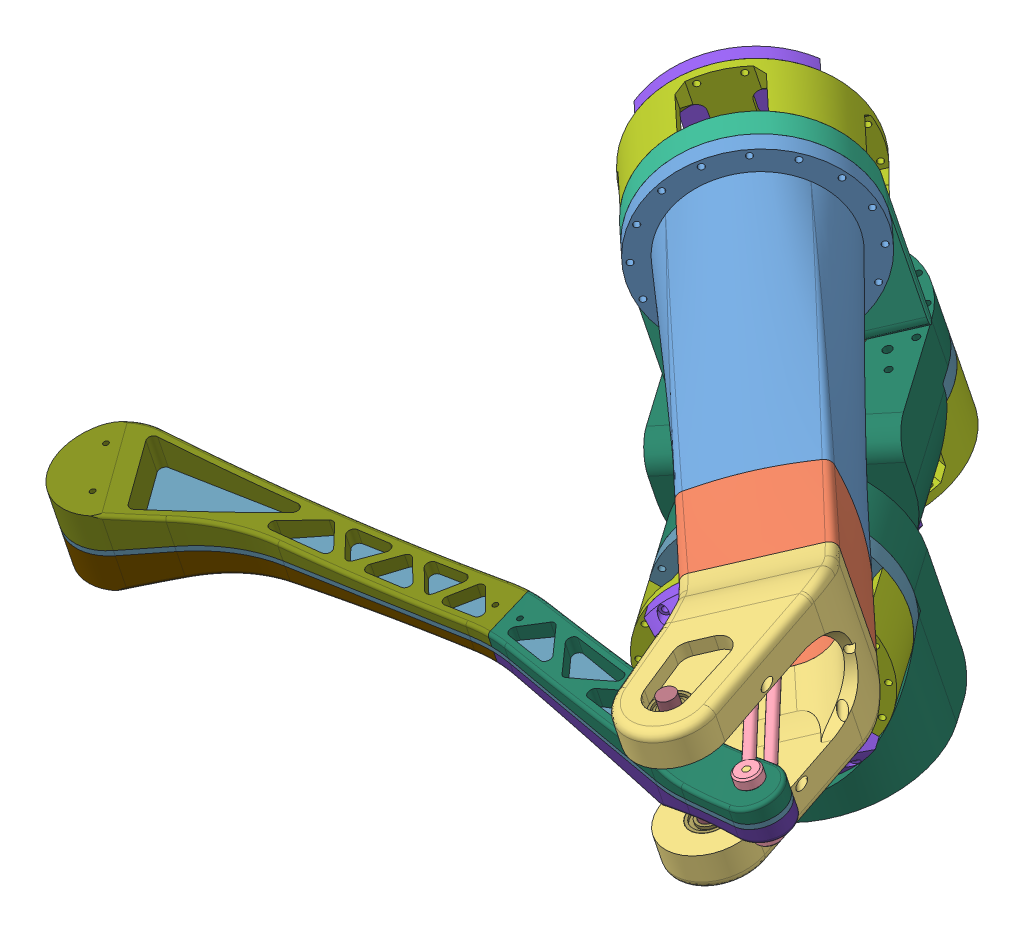
SolidWorks assembly Leg, configuration Default. Lengths in mm. (continued)
Components (placement in the parent): (continued)
- Cycloidal _v3-2: Cycloidal _v3 [Default] at (146.1775 22.9675 470.2476) x (0.670066 -0.524344 -0.525427) z (0.511404 0.83914 -0.185227) size (173.36 87.57 173.15) (continued)
  - foc-motor-controller.step-1: foc-motor-controller.step [Default] at (47.4677 32.6574 89.6282) x (0.701413 0.00028 0.712755) z (0.000399 -1 0) size (57.23 50 8.13) (continued)
    - C_1206_3216Metric.step-13: C_1206_3216Metric.step [Default] at (4 11 1.595) x (0 1 0) z (0 0 1) size (3.2 1.6 1.6)
    - R_0603_1608Metric.step-20: R_0603_1608Metric.step [Default] at (16 -17.8 1.595) x (0 1 0) z (0 0 1) size (1.6 0.8 0.45)
    - Texas_S-PVSON-N8.step-1: Texas_S-PVSON-N8.step [Default] at (-14.4105 -13.7 1.595) x (-1 0 0) z (0 0 1) size (3 2.98 0.92)
    - C_1206_3216Metric.step-14: C_1206_3216Metric.step [Default] at (21 -2.9 1.595) x (0.707107 -0.707107 0) z (0 0 1) size (3.2 1.6 1.6)
    - C_0603_1608Metric.step-24: C_0603_1608Metric.step [Default] at (-5.9 -16.6 1.595) x (0 1 0) z (0 0 1) size (1.6 0.8 0.8)
    - C_0603_1608Metric.step-25: C_0603_1608Metric.step [Default] at (-3.1 -14.1 1.595) size (1.6 0.8 0.8)
    - R_0603_1608Metric.step-21: R_0603_1608Metric.step [Default] at (7.2 -7.375 1.595) x (0 -1 0) z (0 0 1) size (1.6 0.8 0.45)
    - C_1206_3216Metric.step-15: C_1206_3216Metric.step [Default] at (-0.7 11 1.595) x (0 1 0) z (0 0 1) size (3.2 1.6 1.6)
    - LQFP-64_10x10mm_P0.5mm.step-1: LQFP-64_10x10mm_P0.5mm.step [Default] at (-7 -4.5 1.595) x (-1 0 0) z (0 0 1) size (12 12 1.5)
    - C_0805_2012Metric.step-2: C_0805_2012Metric.step [Default] at (23.35 -17 1.595) x (-1 0 0) z (0 0 1) size (2 1.25 1.25)
    - C_0603_1608Metric.step-26: C_0603_1608Metric.step [Default] at (10.8 -16.8 1.595) x (0 -1 0) z (0 0 1) size (1.6 0.8 0.8)
    - R_0603_1608Metric.step-22: R_0603_1608Metric.step [Default] at (17.5 -17.8 1.595) x (0 -1 0) z (0 0 1) size (1.6 0.8 0.45)
    - C_1206_3216Metric.step-16: C_1206_3216Metric.step [Default] at (20.3 11 1.595) x (0 1 0) z (0 0 1) size (3.2 1.6 1.6)
    - R_0603_1608Metric.step-23: R_0603_1608Metric.step [Default] at (9.2 -16.8 1.595) x (0 -1 0) z (0 0 1) size (1.6 0.8 0.45)
    - C_1206_3216Metric.step-17: C_1206_3216Metric.step [Default] at (-10 11 1.595) x (0 1 0) z (0 0 1) size (3.2 1.6 1.6)
    - R_0603_1608Metric.step-24: R_0603_1608Metric.step [Default] at (17.8 -15.2 1.595) size (1.6 0.8 0.45)
    - C_1206_3216Metric.step-18: C_1206_3216Metric.step [Default] at (19.9 2.6 1.595) x (-0.707107 0.707107 0) z (0 0 1) size (3.2 1.6 1.6)
    - C_0603_1608Metric.step-27: C_0603_1608Metric.step [Default] at (13.4 -7.375 1.595) x (0 -1 0) z (0 0 1) size (1.6 0.8 0.8)
    - R_0603_1608Metric.step-25: R_0603_1608Metric.step [Default] at (8.7 -7.375 1.595) x (0 -1 0) z (0 0 1) size (1.6 0.8 0.45)
    - PQFN-8-EP_6x5mm_P1.27mm_Generic.step-1: PQFN-8-EP_6x5mm_P1.27mm_Generic.step [Default] at (4.9 14.4 -0.085) x (0 1 0) z (0 0 -1) size (6.15 5.15 1.09)
    - C_0805_2012Metric.step-3: C_0805_2012Metric.step [Default] at (-3 8.9 -0.085) x (0 1 0) z (0 0 -1) size (2 1.25 1.25)
    - C_0603_1608Metric.step-28: C_0603_1608Metric.step [Default] at (1.5 -4.3 -0.085) x (0 1 0) z (0 0 -1) size (1.6 0.8 0.8)
    - R_2512_6332Metric.step-1: R_2512_6332Metric.step [Default] at (2.1 8.6 -0.085) x (-1 0 0) z (0 0 -1) size (6.3 3.2 0.6)
    - C_0805_2012Metric.step-4: C_0805_2012Metric.step [Default] at (18.8 8.9 -0.085) x (0 1 0) z (0 0 -1) size (2 1.25 1.25)
    - C_0805_2012Metric.step-5: C_0805_2012Metric.step [Default] at (-5.2 8.901 -0.085) x (0 1 0) z (0 0 -1) size (2 1.25 1.25)
    - PQFN-8-EP_6x5mm_P1.27mm_Generic.step-2: PQFN-8-EP_6x5mm_P1.27mm_Generic.step [Default] at (16.9 14.6 -0.085) x (0 -1 0) z (0 0 -1) size (6.15 5.15 1.09)
    - PQFN-8-EP_6x5mm_P1.27mm_Generic.step-3: PQFN-8-EP_6x5mm_P1.27mm_Generic.step [Default] at (-1.1 14.6 -0.085) x (0 -1 0) z (0 0 -1) size (6.15 5.15 1.09)
    - R_0603_1608Metric.step-26: R_0603_1608Metric.step [Default] at (8.2 8.8 -0.085) x (0 1 0) z (0 0 -1) size (1.6 0.8 0.45)
    - R_2512_6332Metric.step-2: R_2512_6332Metric.step [Default] at (-10.3 8.601 -0.085) x (1 0 0) z (0 0 -1) size (6.3 3.2 0.6)
    - TSSOP-16_4.4x5mm_P0.65mm.step-1: TSSOP-16_4.4x5mm_P0.65mm.step [Default] at (0 0 -0.085) x (-1 0 0) z (0 0 -1) size (6.4 5 1.1)
    - C_0603_1608Metric.step-29: C_0603_1608Metric.step [Default] at (0 -4.25 -0.085) x (0 1 0) z (0 0 -1) size (1.6 0.8 0.8)
    - PQFN-8-EP_6x5mm_P1.27mm_Generic.step-4: PQFN-8-EP_6x5mm_P1.27mm_Generic.step [Default] at (10.9 14.4 -0.085) x (0 1 0) z (0 0 -1) size (6.15 5.15 1.09)
    - R_2512_6332Metric.step-3: R_2512_6332Metric.step [Default] at (13.7 8.6 -0.085) x (1 0 0) z (0 0 -1) size (6.3 3.2 0.6)
    - PQFN-8-EP_6x5mm_P1.27mm_Generic.step-5: PQFN-8-EP_6x5mm_P1.27mm_Generic.step [Default] at (-13.1 14.401 -0.085) x (0 1 0) z (0 0 -1) size (6.15 5.15 1.09)
    - C_0603_1608Metric.step-30: C_0603_1608Metric.step [Default] at (-1.5 -4.3 -0.085) x (0 -1 0) z (0 0 -1) size (1.6 0.8 0.8)
    - PQFN-8-EP_6x5mm_P1.27mm_Generic.step-6: PQFN-8-EP_6x5mm_P1.27mm_Generic.step [Default] at (-7.1 14.601 -0.085) x (0 -1 0) z (0 0 -1) size (6.15 5.15 1.09)
    - foc-motor-controller_PCB.step-1: foc-motor-controller_PCB.step [Default] at origin size (50 50 1.51)
  - hex nut style 1 gradeab_iso-1: hex nut style 1 gradeab_iso [ISO - 4032 - M3 - W - N] at (47.7115 32.6575 59.2236) x (1 0.000399 0) z (0.000399 -1 0) size (5.5 6.35 2.4)
  - Cycloidal_Discs_8308-1: Cycloidal_Discs_8308 [Default] at (-11.9184 124.164 51.5043) x (0.028527 0.000011 0.999593) z (0.999593 0.000399 -0.028527) size (79.25 5 79.73)
    - Cycloidal_Discs-1: Cycloidal_Discs [Default] at (38.3081 39.5303 58.0959) size (79.25 5 79.73)
  - Cycloidal_Discs_8308-2: Cycloidal_Discs_8308 [Default] at (62.1667 47.133 159.1742) x (-0.931329 -0.000371 -0.364178) z (0.364178 0.000145 -0.931329) size (79.25 5 79.73)
    - Cycloidal_Discs-1: Cycloidal_Discs [Default] at (38.3081 39.5303 58.0959) size (79.25 5 79.73)
  - Motor_Cover_v2-2: Motor_Cover_v2 [Default] at (47.4667 35.0574 89.6282) x (0.999968 0.000399 0.00802) z (-0.00802 -0.000003 0.999968) size (115 34.6 115)
  - driver_cover-1: driver_cover [Default] at (47.4667 35.0574 89.6282) x (0.702656 0.00028 0.711529) z (0.711529 0.000284 -0.702656) size (81.32 15 115)
  - Cover_new-1: Cover_new [Default] at (47.4437 92.6574 89.6282) x (0.701413 0.00028 0.712755) z (-0.712755 -0.000284 0.701413) size (115 87.5 130)
  - Output_Shaft-2: Output_Shaft [Default] at (47.4437 92.6574 89.6282) x (0.572675 0.000228 0.819783) z (-0.819783 -0.000327 0.572675) size (70 14 70)
  - radial ball bearing_68_iso-47: radial ball bearing_68_iso [ISO 15 RBB - 289 - 14,SI,NC,14_68] at (61.9924 89.1632 109.081) x (0.000399 -1 0) z (-0.055662 -0.000022 0.99845) size (5 17 17)
  - radial ball bearing_68_iso-48: radial ball bearing_68_iso [ISO 15 RBB - 289 - 14,SI,NC,14_68] at (59.3269 82.1622 107.722) x (0.000399 -1 0) z (-0.055662 -0.000022 0.99845) size (5 17 17)
  - m4x14-1: m4x14 [Default] at (47.0925 68.4573 134.6267) x (0.999623 0.000399 0.027466) z (-0.027466 -0.000011 0.999623) size (8 15.2 8)
  - M3x20-1: M3x20 [Default] at (43.4726 96.3558 90.1203) x (-0.837193 -0.000334 -0.546908) z (-0.546908 -0.000218 0.837193) size (6 21.2 6)
  - M3x10-1: M3x10 [Default] at (36.5111 25.853 142.5044) x (0.424034 0.000169 -0.905646) z (0.905646 0.000361 0.424034) size (6 11.2 6)
  - m3x60-1: m3x60 [Default] at (17.1068 35.0453 134.2855) x (-0.837193 -0.000334 -0.546908) z (-0.546908 -0.000218 0.837193) size (5.3 63 5.3)
  - m6-1: m6 [Default] at (60.6129 98.6627 108.4832) x (-0.153131 -0.000061 0.988206) z (0.988206 0.000394 0.153131) size (6 16 6)
- Output_2-1: Output_2 [Default] at (116.2562 155.7127 287.3925) x (0.968552 0.057949 0.241968) z (-0.218652 -0.265847 0.938891) size (60 8 60)
- Output_2-2: Output_2 [Default] at (166.4156 88.7259 340.149) x (0.781948 -0.281597 -0.556112) z (0.314314 0.948544 -0.038357) size (60 8 60)
- radial ball bearing_68_iso-5: radial ball bearing_68_iso [ISO 15 RBB - 1910 - 10,SI,NC,10_68] at (346.2156 224.7988 595.0703) x (-0.118734 0.962272 0.244816) z (0.823708 -0.042219 0.56544) size (6 22 22)
- m4_Shaft-1: m4_Shaft [Default] at (392.2849 177.9376 583.0745) x (0.992606 0.121291 0.004661) z (0.025209 -0.243559 0.969558) size (4 39 4)
- radial ball bearing_68_iso-6: radial ball bearing_68_iso [ISO 15 RBB - 1910 - 10,SI,NC,10_68] at (354.2896 159.3643 578.4228) x (-0.118734 0.962272 0.244816) z (0.248305 0.267502 -0.931014) size (6 22 22)
- radial ball bearing_68_iso-7: radial ball bearing_68_iso [ISO 15 RBB - 1910 - 10,SI,NC,10_68] at (353.5772 165.1379 579.8917) x (-0.118734 0.962272 0.244816) z (0.248305 0.267502 -0.931014) size (6 22 22)
Mates (geometry in assembly coordinates):
- Concentric7: concentric aligned: cylinder of ball_screw-1 through (273.972 214.2064 462.7873) axis (-0.729494 0.082727 -0.678966) radius 5; cylinder of ball_screw_slider-1 through (247.2728 217.2341 437.9374) axis (-0.729494 0.082727 -0.678966) radius 5
- Concentric8: concentric aligned: cylinder of ball_screw_slider-1 through (247.2728 217.2341 437.9374) axis (-0.729494 0.082727 -0.678966) radius 14; cylinder of connection_rod_base-1 through (226.1175 219.6332 418.2474) axis (-0.729494 0.082727 -0.678966) radius 14
- Coincident10: coincident anti-aligned: plane of ball_screw_slider-1 through (223.929 219.8814 416.2105) normal (0.729494 -0.082727 0.678966); plane of connection_rod_base-1 through (223.929 219.8814 416.2105) normal (-0.729494 0.082727 -0.678966)
- Concentric9: concentric aligned: cylinder of Link_Rod-1 through (387.6543 215.4662 592.6223) axis (0.118734 -0.962272 -0.244816) radius 7; cylinder of Link_Rod-2 through (391.4538 184.6735 584.7882) axis (0.118734 -0.962272 -0.244816) radius 7
- Parallel2: parallel aligned: plane of ball_screw_slider-1 through (219.874 206.1091 407.1065) normal (0.118734 -0.962272 -0.244816); plane of connection_rod_base-1 through (228.789 197.9821 412.739) normal (0.118734 -0.962272 -0.244816)
- Concentric13: concentric anti-aligned: cylinder of ball_screw-1 through (149.2285 228.3527 346.6841) axis (0.729494 -0.082727 0.678966) radius 4; cylinder of Shaft Coupler D25L30 8x8.step-1/8x8_Flexible_Spider_Shaft_Coupling.step-1/Coupler L.step-1 through (154.335 227.7736 351.4369) axis (-0.729494 0.082727 -0.678966) radius 4
- Coincident14: coincident anti-aligned: plane of ball_screw-1 through (157.9825 227.36 354.8317) normal (-0.729494 0.082727 -0.678966); plane of Shaft Coupler D25L30 8x8.step-1/8x8_Flexible_Spider_Shaft_Coupling.step-1/Coupler L.step-1 through (157.9825 227.36 354.8317) normal (0.729494 -0.082727 0.678966)
- Concentric14: concentric anti-aligned: cylinder of Shaft Coupler D25L30 8x8.step-1/8x8_Flexible_Spider_Shaft_Coupling.step-1/Coupler R.step-1 through (136.0926 229.8406 334.468) axis (0.729494 -0.082727 0.678966) radius 4; cylinder of m8-1 through (144.8466 228.8478 342.6156) axis (-0.729494 0.082727 -0.678966) radius 4
- Coincident15: coincident anti-aligned: plane of Shaft Coupler D25L30 8x8.step-1/8x8_Flexible_Spider_Shaft_Coupling.step-1/Coupler R.step-1 through (136.0926 229.8406 334.468) normal (-0.729494 0.082727 -0.678966); plane of m8-1 through (136.0926 229.8406 334.468) normal (0.729494 -0.082727 0.678966)
- Coincident17: coincident aligned: plane of m8-1 through (131.205 230.3948 329.9189) normal (-0.729494 0.082727 -0.678966); plane of Output_Shaft_holder-1 through (131.21 230.396 329.9137) normal (-0.729494 0.082727 -0.678966)
- Concentric21: concentric anti-aligned: cylinder of m10-1 through (344.9096 235.3838 597.7633) axis (0.118734 -0.962272 -0.244816) radius 5; cylinder of radial ball bearing_68_iso-4 through (349.3784 199.1663 588.549) axis (-0.118734 0.962272 0.244816) radius 5
- Concentric39: concentric anti-aligned: cylinder of m10-1 through (344.9096 235.3838 597.7633) axis (0.118734 -0.962272 -0.244816) radius 5; cylinder of radial ball bearing_68_iso-3 through (357.6898 131.8072 571.4119) axis (-0.118734 0.962272 0.244816) radius 5
- Concentric42: concentric aligned: cylinder of m10-1 through (344.9096 235.3838 597.7633) axis (0.118734 -0.962272 -0.244816) radius 5; cylinder of Leg_Lower-1/Leg_Lower_out_left_1-1 through (347.6998 212.7704 592.0101) axis (0.118734 -0.962272 -0.244816) radius 5
- Concentric43: concentric anti-aligned: circle of Link_Rod-1; cylinder of Leg_Lower-1/Leg_Lower_out_left_1-1 through (387.4168 217.3907 593.112) axis (0.118734 -0.962272 -0.244816) radius 2
- Concentric48: concentric anti-aligned: cylinder of ball_screw-1 through (279.0785 213.6273 467.5401) axis (-0.729494 0.082727 -0.678966) radius 3; cylinder of radial ball bearing_68_iso-1 through (260.7408 215.7068 450.4726) axis (0.729494 -0.082727 0.678966) radius 3
- Coincident73: coincident aligned: plane of ball_screw-1 through (273.972 214.2064 462.7873) normal (0.729494 -0.082727 0.678966); circle of radial ball bearing_68_iso-1
- Concentric50: concentric anti-aligned: cylinder of m10-1 through (344.9096 235.3838 597.7633) axis (0.118734 -0.962272 -0.244816) radius 5; cylinder of Leg_upper-1/kfe-1 through (336.5659 147.7875 591.2628) axis (-0.234603 0.920392 0.312795) radius 11
- Coincident75: coincident aligned: plane of m10-1 through (344.9096 235.3838 597.7633) normal (-0.118734 0.962272 0.244816); plane of Leg_upper-1/kfe-1 through (301.985 249.6244 553.4023) normal (-0.234603 0.920392 0.312795)
- Coincident76: coincident aligned: plane of Leg_Lower-1/Leg_Lower_in-1 through (350.2526 192.0815 586.7465) normal (-0.118734 0.962272 0.244816); plane of Leg_upper-1/kfe-1 through (312.5421 208.2067 539.3265) normal (-0.234603 0.920392 0.312795)
- Coincident77: coincident aligned: plane of m10-1 through (355.5956 148.7793 575.7298) normal (0.118734 -0.962272 -0.244816); plane of radial ball bearing_68_iso-3 through (364.4403 149.237 578.2202) normal (0.118734 -0.962272 -0.244816)
- Concentric53: concentric aligned: cylinder of Output_Shaft_holder-1 through (134.8575 229.9824 333.3085) axis (-0.729494 0.082727 -0.678966) radius 20; cylinder of Leg_upper-1/leg_upper_infront_1-1 through (138.505 229.5688 336.7033) axis (-0.729494 0.082727 -0.678966) radius 27
- Coincident82: coincident aligned: plane of Output_Shaft_holder-1 through (131.21 230.396 329.9137) normal (-0.729494 0.082727 -0.678966); plane of Leg_upper-1/leg_upper_infront_1-1 through (131.21 230.396 329.9137) normal (-0.729494 0.082727 -0.678966)
- Concentric54: concentric aligned: cylinder of ball_screw-1 through (273.972 214.2064 462.7873) axis (-0.729494 0.082727 -0.678966) radius 5; cylinder of Leg_upper-1/leg_upper_infront_1-1 through (138.505 229.5688 336.7033) axis (-0.729494 0.082727 -0.678966) radius 27
- Concentric56: concentric anti-aligned: cylinder of Output_Shaft_holder-1 through (145.3434 229.0658 321.9306) axis (-0.729494 0.082727 -0.678966) radius 2; cylinder of m4x14-1 through (134.0362 230.348 311.4066) axis (0.729494 -0.082727 0.678966) radius 2
- Parallel6: parallel anti-aligned: plane of Output_Shaft_holder-1 through (134.8575 229.9824 333.3085) normal (0.729494 -0.082727 0.678966); plane of m4x14-1 through (144.2491 229.1899 320.9122) normal (-0.729494 0.082727 -0.678966)
- Coincident91: coincident anti-aligned: plane of Output_Shaft_holder-1 through (144.2491 229.1899 320.9122) normal (0.729494 -0.082727 0.678966); plane of m4x14-1 through (144.2491 229.1899 320.9122) normal (-0.729494 0.082727 -0.678966)
- Concentric57: concentric anti-aligned: cylinder of Leg_upper-1/leg_upper_infront_1-1 through (138.505 229.5688 336.7033) axis (-0.729494 0.082727 -0.678966) radius 57.5; cylinder of kfe_bldc-1/cover-1 through (120.2676 231.6369 319.7292) axis (0.729494 -0.082727 0.678966) radius 57.5
- Coincident92: coincident anti-aligned: plane of Leg_upper-1/leg_upper_infront_1-1 through (131.21 230.396 329.9137) normal (-0.729494 0.082727 -0.678966); plane of kfe_bldc-1/cover-1 through (131.21 230.396 329.9137) normal (0.729494 -0.082727 0.678966)
- Concentric59: concentric aligned: cylinder of Cycloidal _v3-2/Cover_new-1 through (166.4156 88.7259 340.149) axis (0.538297 -0.1448 0.830222) radius 57.5; cylinder of Output_2-2 through (162.1092 89.8843 333.5072) axis (0.538297 -0.1448 0.830222) radius 30
- Coincident93: coincident anti-aligned: plane of Cycloidal_v3-2/Output_Shaft-1 through (186.2868 98.7261 325.3992) normal (-0.772321 0.018927 -0.63495); plane of Output_2-2 through (166.4156 88.7259 340.149) normal (0.538297 -0.1448 0.830222)
- Concentric60: concentric aligned: cylinder of Cycloidal _v3-1/Cover_new-1 through (116.2562 155.7127 287.3925) axis (0.118734 -0.962272 -0.244816) radius 57.5; cylinder of Output_2-1 through (115.3063 163.4109 289.351) axis (0.118734 -0.962272 -0.244816) radius 30
- Concentric61: concentric anti-aligned: circle of kfe_bldc-1/cover-1; circle of Output_2-1
- Concentric62: concentric anti-aligned: circle of kfe_bldc-1/cover-1; circle of Output_2-1
- Coincident95: coincident anti-aligned: plane of kfe_bldc-1/cover-1 through (101.0861 145.7268 351.9631) normal (0.118734 -0.962272 -0.244816); plane of Output_2-1 through (115.3063 163.4109 289.351) normal (-0.118734 0.962272 0.244816)
- Coincident97: coincident anti-aligned: circle of radial ball bearing_68_iso-1; plane of Leg_upper-1/leg_upper_infront_2-1 through (147.273 -11.2949 571.4394) normal (-0.729494 0.082727 -0.678966)
- Concentric65: concentric anti-aligned: circle of radial ball bearing_68_iso-1; cylinder of Leg_upper-1/leg_upper_infront_2-1 through (281.2669 213.3791 469.577) axis (-0.729494 0.082727 -0.678966) radius 6.5
- Concentric67: concentric anti-aligned: cylinder of m10-1 through (344.9096 235.3838 597.7633) axis (0.118734 -0.962272 -0.244816) radius 5; cylinder of radial ball bearing_68_iso-5 through (348.666 204.9399 590.0179) axis (-0.118734 0.962272 0.244816) radius 5
- Coincident99: coincident anti-aligned: plane of radial ball bearing_68_iso-4 through (340.793 219.0285 602.867) normal (-0.118734 0.962272 0.244816); plane of radial ball bearing_68_iso-5 through (342.8016 220.0842 599.6916) normal (0.118734 -0.962272 -0.244816)
- Coincident100: coincident aligned: plane of Leg_upper-1/kfe-1 through (303.8618 242.2612 550.8999) normal (-0.234603 0.920392 0.312795); circle of radial ball bearing_68_iso-5
- Concentric70: concentric aligned: cylinder of Link_Rod-1 through (250.7934 235.3366 448.143) axis (0.118734 -0.962272 -0.244816) radius 2; cylinder of Link_Rod-2 through (254.5929 204.5439 440.3089) axis (0.118734 -0.962272 -0.244816) radius 2
- Coincident103: coincident anti-aligned: line of connection_rod_base-1 through (250.7934 235.3366 448.143) axis (-0.118734 0.962272 0.244816); line of Link_Rod-1 through (250.9121 234.3744 447.8982) axis (0.118734 -0.962272 -0.244816)
- Coincident104: coincident anti-aligned: plane of connection_rod_base-1 through (250.7934 235.3366 448.143) normal (0.118734 -0.962272 -0.244816); plane of Link_Rod-1 through (250.7934 235.3366 448.143) normal (-0.118734 0.962272 0.244816)
- Coincident105: coincident aligned: plane of connection_rod_base-1 through (255.424 197.808 438.5952) normal (-0.118734 0.962272 0.244816); circle of Link_Rod-2
- Concentric71: concentric anti-aligned: cylinder of m10-1 through (344.9096 235.3838 597.7633) axis (0.118734 -0.962272 -0.244816) radius 5; cylinder of Leg_upper-1/leg_upper_infront_2_kfe-1 through (355.5956 148.7793 575.7298) axis (-0.118734 0.962272 0.244816) radius 11
- Coincident106: coincident aligned: plane of m10-1 through (344.9096 235.3838 597.7633) normal (-0.118734 0.962272 0.244816); plane of Leg_upper-1/leg_upper_infront_2_kfe-1 through (125.867 273.6983 340.9304) normal (-0.118734 0.962272 0.244816)
- Coincident107: coincident aligned: plane of Leg_upper-1/leg_upper_infront_2_kfe-1 through (126.8169 266.0001 338.9719) normal (-0.118734 0.962272 0.244816); circle of radial ball bearing_68_iso-5
- Coincident115: coincident aligned: plane of connection_rod_base-1 through (223.929 219.8814 416.2105) normal (-0.118734 0.962272 0.244816); plane of Leg_Lower-1/Leg_Lower_in-1 through (350.2526 192.0815 586.7465) normal (-0.118734 0.962272 0.244816)
- Concentric73: concentric anti-aligned: cylinder of Leg_upper-1/leg_upper_infront_1-1 through (125.1202 277.8023 356.9611) axis (-0.729494 0.082727 -0.678966) radius 1.75; cylinder of kfe_bldc-1/cover-1 through (106.8829 279.8705 339.9869) axis (0.729494 -0.082727 0.678966) radius 1.5
- Concentric74: concentric aligned: line of Link_Rod-1 through (387.6543 215.4662 592.6223) axis (0.118734 -0.962272 -0.244816); cylinder of m4_Shaft-1 through (387.6543 215.4662 592.6223) axis (0.118734 -0.962272 -0.244816) radius 2
- Coincident118: coincident aligned: plane of Link_Rod-1 through (387.6543 215.4662 592.6223) normal (-0.118734 0.962272 0.244816); plane of m4_Shaft-1 through (387.6543 215.4662 592.6223) normal (-0.118734 0.962272 0.244816)
- Concentric75: concentric aligned: cylinder of radial ball bearing_68_iso-6 through (356.7399 139.5054 573.3704) axis (-0.118734 0.962272 0.244816) radius 11; cylinder of radial ball bearing_68_iso-7 through (356.0275 145.279 574.8393) axis (-0.118734 0.962272 0.244816) radius 11
- Coincident119: coincident anti-aligned: plane of radial ball bearing_68_iso-6 through (364.2201 162.7835 582.0537) normal (-0.118734 0.962272 0.244816); plane of radial ball bearing_68_iso-7 through (362.778 162.7088 581.6477) normal (0.118734 -0.962272 -0.244816)
- Coincident120: coincident aligned: plane of Leg_upper-1/leg_upper_infront_2_kfe-1 through (421.9635 215.3175 428.0773) normal (-0.118734 0.962272 0.244816); plane of radial ball bearing_68_iso-7 through (363.5077 168.5571 583.5226) normal (-0.118734 0.962272 0.244816)
- Concentric76: concentric anti-aligned: cylinder of m10-1 through (344.9096 235.3838 597.7633) axis (0.118734 -0.962272 -0.244816) radius 5; cylinder of radial ball bearing_68_iso-7 through (356.0275 145.279 574.8393) axis (-0.118734 0.962272 0.244816) radius 5
- Coincident121: coincident anti-aligned: plane of Cycloidal _v3-1/Output_Shaft-2 through (116.2562 155.7127 287.3925) normal (-0.118734 0.962272 0.244816); plane of Output_2-1 through (116.2562 155.7127 287.3925) normal (0.118734 -0.962272 -0.244816)
- Coincident122: coincident anti-aligned: plane of Cycloidal _v3-2/Output_Shaft-2 through (166.4156 88.7259 340.149) normal (-0.538297 0.1448 -0.830222); plane of Output_2-2 through (166.4156 88.7259 340.149) normal (0.538297 -0.1448 0.830222)
- Concentric78: concentric anti-aligned: cylinder of Cycloidal _v3-1/Cover_new-1 through (133.0049 121.4743 276.5839) axis (0.538297 -0.1448 0.830222) radius 2.25; circle of Output_2-2
- Concentric80: concentric aligned: line of Cycloidal _v3-1/Cover_new-1 through (149.497 69.5158 326.0872) axis (0.538297 -0.1448 0.830222); cylinder of Output_2-2 through (154.88 68.0678 334.3894) axis (0.538297 -0.1448 0.830222) radius 2.1
- Coincident125: coincident anti-aligned: plane of Cycloidal _v3-1/Cover_new-1 through (108.97 118.4972 372.9519) normal (0.538297 -0.1448 0.830222); plane of Output_2-2 through (162.1092 89.8843 333.5072) normal (-0.538297 0.1448 -0.830222)
- Parallel9: parallel anti-aligned: plane of Cycloidal _v3-1/Cover_new-1 through (116.2562 155.7127 287.3925) normal (-0.118734 0.962272 0.244816); plane of Cycloidal _v3-2/Cover_new-1 through (230.535 30.1797 305.2272) normal (0.118734 -0.962272 -0.244816)
